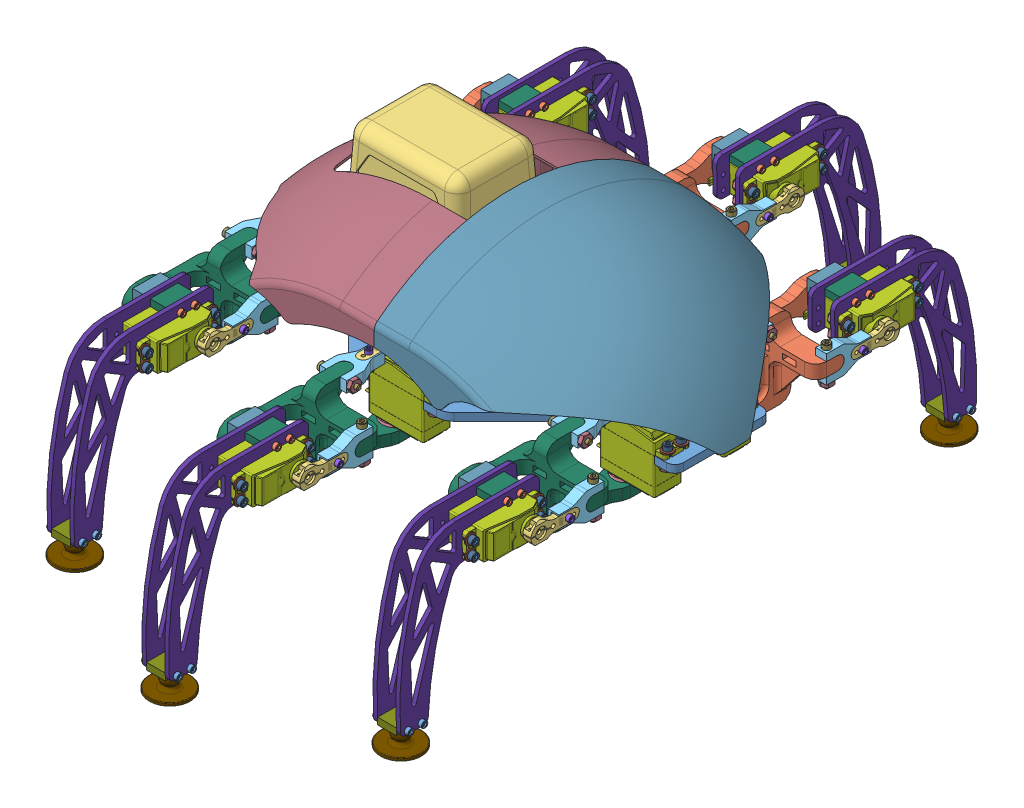
SolidWorks assembly Hexapod_(Small), configuration Défaut. Lengths in mm.
Overall size (338.69 208.02 531.29).
425 component instances, 33 part files, 134 mates.
Components (placement in the parent):
- Body_(Small)-5: Body_(Small) [Default] at (-310 -5.6 15.2) x (1 0 0) z (0 1 0) size (310 170.8 5.6)
- Foot+Femur_(Mirror)-6: Foot+Femur_(Mirror) [Défaut] at (-15 -28 -0.2) x (0 0 1) z (-1 0 0) size (215.83 135.72 63.38)
  - Femur_(Mirror)-1: Femur_(Mirror) [Défaut] at origin size (137.38 61.64 60.79) (flexible)
    - Joint_(Femur_to_tibia)_(Mirror)-2: Joint_(Femur_to_tibia)_(Mirror) [Défaut] at (-66.2306 29.5 32.9516) x (0.999952 0 0.00979) z (-0.00979 0 0.999952) size (122 58.8 58.8)
    - Horn-4: Horn [Défaut] at (-10.2 48.8 30.1) x (-0.999952 0 -0.00979) z (0 1 0) size (35.39 15.87 6)
    - Bearing_mount_(Femur)-2: Bearing_mount_(Femur) [Default] at (2.5 22 30.1) x (1 0 0) z (0 -1 0) size (35.3 20.2 31)
    - Horn_attachment-4: Horn_attachment [Défaut] at (-38.1987 44.8 29.8259) x (0.999952 0 0.00979) z (0 1 0) size (33 20 8)
    - Bearing-4: Bearing [Default] at (-10.2 -6.7498 30.1) x (0.165905 0 -0.986142) z (0.986142 0 0.165905) size (13.87 4.75 13.87)
    - DS3225MG-4: DS3225MG [Default] at (-10.2 45.8 30.1) x (0 0 -1) z (0 1 0) size (57.25 20.4 45.91)
    - HX-SHCS 0.112-40x0.4375x0.4375-N-1: HX-SHCS 0.112-40x0.4375x0.4375-N [HX-SHCS 0.112-40x0.4375x0.4375-N] at (-30.199 51.6448 29.9042) x (0 -1 0) z (-0.508455 0 0.861089) size (13.96 4.65 4.65)
    - MSHXNUT 0.112-40-D-N-1: MSHXNUT 0.112-40-D-N [MSHXNUT 0.112-40-D-N] at (-30.199 40.8 29.9042) x (-0.491498 0 -0.870879) z (0 1 0) size (6.35 7.33 2.49)
    - HX-SHCS 0.138-32x0.5x0.5-N-1: HX-SHCS 0.138-32x0.5x0.5-N [HX-SHCS 0.138-32x0.5x0.5-N] at (-15.2 35.772 -4.7) x (0 -1 0) z (0.866025 0 -0.5) size (16.21 5.74 5.74)
    - Narrow FW 0.138-1: Narrow FW 0.138 [Narrow FW 0.138] at (-15.2 31.2 -4.7) x (0 -1 0) z (-0.829316 0 -0.55878) size (0.81 7.92 7.92)
    - HX-SHCS 0.138-32x0.5x0.5-N-2: HX-SHCS 0.138-32x0.5x0.5-N [HX-SHCS 0.138-32x0.5x0.5-N] at (-15.2 35.772 44.9) x (0 -1 0) z (0.866025 0 -0.5) size (16.21 5.74 5.74)
    - HX-SHCS 0.138-32x0.5x0.5-N-3: HX-SHCS 0.138-32x0.5x0.5-N [HX-SHCS 0.138-32x0.5x0.5-N] at (-5.2 35.772 -4.7) x (0 -1 0) z (0.866025 0 -0.5) size (16.21 5.74 5.74)
    - HX-SHCS 0.138-32x0.5x0.5-N-4: HX-SHCS 0.138-32x0.5x0.5-N [HX-SHCS 0.138-32x0.5x0.5-N] at (-5.2 35.772 44.9) x (0 -1 0) z (0.866025 0 -0.5) size (16.21 5.74 5.74)
    - Narrow FW 0.138-2: Narrow FW 0.138 [Narrow FW 0.138] at (-15.2 31.2 44.9) x (0 -1 0) z (-0.829316 0 -0.55878) size (0.81 7.92 7.92)
    - Narrow FW 0.138-3: Narrow FW 0.138 [Narrow FW 0.138] at (-5.2 31.2 -4.7) x (0 -1 0) z (-0.829316 0 -0.55878) size (0.81 7.92 7.92)
    - Narrow FW 0.138-4: Narrow FW 0.138 [Narrow FW 0.138] at (-5.2 31.2 44.9) x (0 -1 0) z (-0.829316 0 -0.55878) size (0.81 7.92 7.92)
    - HX-SHCS 0.138-32x1x1-N-1: HX-SHCS 0.138-32x1x1-N [HX-SHCS 0.138-32x1x1-N] at (-52.3302 44.8 43.1934) x (0.00979 0 -0.999952) z (-0.865984 0.5 -0.008479) size (28.91 5.74 5.74)
    - MSHXNUT 0.138-32-D-N-1: MSHXNUT 0.138-32-D-N [MSHXNUT 0.138-32-D-N] at (-52.0717 44.8 16.7938) x (0.865984 -0.5 0.008479) z (0.00979 0 -0.999952) size (7.92 9.15 2.9)
  - Foot_(Short)_(Mirror)-1: Foot_(Short)_(Mirror) [Défaut] at (-102.2988 19.1911 38.5987) x (0.999893 -0.010844 0.00979) z (-0.00979 0 0.999952) size (133.45 132 60.64) (flexible)
    - Horn_attachment-2: Horn_attachment [Défaut] at (17.8984 10.5036 -44.8) x (-0.999941 -0.010844 0) z (0 0 -1) size (33 20 8)
    - Bearing-2: Bearing [Default] at (-10.1 10.2 6.7498) x (0.20972 0.977761 0) z (-0.977761 0.20972 0) size (13.87 4.75 13.87)
    - Bearing_mount_(Foot)-2: Bearing_mount_(Foot) [Default] at (-10.1 22.9 -8.1) x (0 1 0) z (0 0 1) size (25.3 20.2 17.1)
    - Link-3: Link [Default] at (-10.1 22.9 -25) x (0 -1 0) z (0 0 1) size (5 20.2 13.9)
    - Horn-2: Horn [Défaut] at (-10.1 10.2 -48.8) x (0.999941 0.010844 0) z (0 0 -1) size (35.39 15.87 6)
    - Joint_(Foot_to_slipper)-4: Joint_(Foot_to_slipper) [Default] at (-82.4457 -87.5 -25) x (0 1 0) z (0 0 1) size (15 20.2 13.9)
    - Foot_(Short)-3: Foot_(Short) [Default] at (-21.5 14 -28) size (102.48 118 3)
    - DS3225MG-2: DS3225MG [Default] at (-10.1 10.2 -45.8) x (-1 0 0) z (0 0 -1) size (57.25 20.4 45.91)
    - Foot_(Short)-4: Foot_(Short) [Default] at (-21.5 14 -11.1) size (102.48 118 3)
    - Slipper-1: Slipper [Défaut] at (-82.4457 -102 -18.05) size (30 10.55 30)
    - HX-SHCS 0.112-40x0.4375x0.4375-N-1: HX-SHCS 0.112-40x0.4375x0.4375-N [HX-SHCS 0.112-40x0.4375x0.4375-N] at (9.8988 10.4169 -51.6448) x (0 0 1) z (0.509362 -0.860552 0) size (13.96 4.65 4.65)
    - MSHXNUT 0.112-40-D-N-1: MSHXNUT 0.112-40-D-N [MSHXNUT 0.112-40-D-N] at (9.8988 10.4169 -40.8) x (-0.509362 0.860552 0) z (0 0 -1) size (6.35 7.33 2.49)
    - HX-SHCS 0.112-40x0.875x0.875-N-1: HX-SHCS 0.112-40x0.875x0.875-N [HX-SHCS 0.112-40x0.875x0.875-N] at (-87.4457 -87.5 -30.8448) x (0 0 1) z (0 1 0) size (25.07 4.65 4.65)
    - MSHXNUT 0.112-40-D-N-2: MSHXNUT 0.112-40-D-N [MSHXNUT 0.112-40-D-N] at (-87.4457 -87.5 -8.1) x (-0.866025 -0.5 0) z (0 0 -1) size (6.35 7.33 2.49)
    - MSHXNUT 0.112-40-D-N-3: MSHXNUT 0.112-40-D-N [MSHXNUT 0.112-40-D-N] at (-77.4457 -87.5 -8.1) x (-0.866025 -0.5 0) z (0 0 -1) size (6.35 7.33 2.49)
    - HX-SHCS 0.112-40x0.875x0.875-N-2: HX-SHCS 0.112-40x0.875x0.875-N [HX-SHCS 0.112-40x0.875x0.875-N] at (-77.4457 -87.5 -30.8448) x (0 0 1) z (0 1 0) size (25.07 4.65 4.65)
    - HX-SHCS 0.112-40x1x0.75-N-3: HX-SHCS 0.112-40x1x0.75-N [HX-SHCS 0.112-40x1x0.75-N] at (-5.1 22.9 -30.8448) x (0 0 1) z (-0.866025 0.5 0) size (28.24 4.65 4.65)
    - HX-SHCS 0.112-40x1x0.75-N-4: HX-SHCS 0.112-40x1x0.75-N [HX-SHCS 0.112-40x1x0.75-N] at (-15.1 22.9 -30.8448) x (0 0 1) z (-0.866025 0.5 0) size (28.24 4.65 4.65)
    - HX-SHCS 0.138-32x0.5x0.5-N-1: HX-SHCS 0.138-32x0.5x0.5-N [HX-SHCS 0.138-32x0.5x0.5-N] at (-44.9 5.2 -35.772) x (0 0 1) z (-0.866025 0.5 0) size (16.21 5.74 5.74)
    - Narrow FW 0.138-1: Narrow FW 0.138 [Narrow FW 0.138] at (-44.9 5.2 -31.2) x (0 0 1) z (0.552023 0.833829 0) size (0.81 7.92 7.92)
    - MSHXNUT 0.138-32-D-N-1: MSHXNUT 0.138-32-D-N [MSHXNUT 0.138-32-D-N] at (-44.9 5.2 -25) x (-0.866025 -0.5 0) z (0 0 -1) size (7.92 9.15 2.9)
    - HX-SHCS 0.138-32x0.5x0.5-N-2: HX-SHCS 0.138-32x0.5x0.5-N [HX-SHCS 0.138-32x0.5x0.5-N] at (4.7 5.2 -35.772) x (0 0 1) z (-0.866025 0.5 0) size (16.21 5.74 5.74)
    - HX-SHCS 0.138-32x0.5x0.5-N-3: HX-SHCS 0.138-32x0.5x0.5-N [HX-SHCS 0.138-32x0.5x0.5-N] at (-44.9 15.2 -35.772) x (0 0 1) z (-0.866025 0.5 0) size (16.21 5.74 5.74)
    - HX-SHCS 0.138-32x0.5x0.5-N-4: HX-SHCS 0.138-32x0.5x0.5-N [HX-SHCS 0.138-32x0.5x0.5-N] at (4.7 15.2 -35.772) x (0 0 1) z (-0.866025 0.5 0) size (16.21 5.74 5.74)
    - Narrow FW 0.138-2: Narrow FW 0.138 [Narrow FW 0.138] at (4.7 5.2 -31.2) x (0 0 1) z (0.552023 0.833829 0) size (0.81 7.92 7.92)
    - Narrow FW 0.138-3: Narrow FW 0.138 [Narrow FW 0.138] at (-44.9 15.2 -31.2) x (0 0 1) z (0.552023 0.833829 0) size (0.81 7.92 7.92)
    - Narrow FW 0.138-4: Narrow FW 0.138 [Narrow FW 0.138] at (4.7 15.2 -31.2) x (0 0 1) z (0.552023 0.833829 0) size (0.81 7.92 7.92)
    - MSHXNUT 0.138-32-D-N-2: MSHXNUT 0.138-32-D-N [MSHXNUT 0.138-32-D-N] at (4.7 5.2 -25) x (-0.866025 -0.5 0) z (0 0 -1) size (7.92 9.15 2.9)
    - MSHXNUT 0.138-32-D-N-3: MSHXNUT 0.138-32-D-N [MSHXNUT 0.138-32-D-N] at (-44.9 15.2 -25) x (-0.866025 -0.5 0) z (0 0 -1) size (7.92 9.15 2.9)
    - MSHXNUT 0.138-32-D-N-4: MSHXNUT 0.138-32-D-N [MSHXNUT 0.138-32-D-N] at (4.7 15.2 -25) x (-0.866025 -0.5 0) z (0 0 -1) size (7.92 9.15 2.9)
  - HX-SHCS 0.138-32x1x1-N-1: HX-SHCS 0.138-32x1x1-N [HX-SHCS 0.138-32x1x1-N] at (-69.8506 43.0052 -5.8857) x (0 -1 0) z (0.861089 0 0.508455) size (28.91 5.74 5.74)
  - MSHXNUT 0.138-32-D-N-1: MSHXNUT 0.138-32-D-N [MSHXNUT 0.138-32-D-N] at (-69.8506 16.6044 -5.8857) x (0.00979 0 -0.999952) z (0 -1 0) size (7.92 9.15 2.9)
- Battery-1: Battery [Défaut] at (-120.5058 65.3901 15.3939) x (0 0 -1) z (-1 0 0) size (64.47 74.3 85.78)
  - MAKITA 4.0AH-1: MAKITA 4.0AH [Défaut] at (0.5853 -29.7874 85.4436) size (64.47 57.15 85.78)
  - MAKITA 4.0AH MOBILE-1: MAKITA 4.0AH MOBILE [Défaut] at (0.5853 -39.3124 91.7936) size (45.84 26.68 66.29)
- arduinoMega-1: arduinoMega [Detailed] at (-199.11 -7.6 14.42) x (0 0 -1) z (-1 0 0) size (108.32 14.5 53.3)
- raspberryPi3B-1: raspberryPi3B [Detailed] at (-109 6.35 15.2) x (-1 0 0) z (0 1 0) size (87.05 58.5 19.5)
- 12Channel PWM-1: 12Channel PWM [Default] at (-145.4 -5.6 15.2) x (-1 0 0) z (0 0 1) size (25.4 7.55 66.7)
- DROK_090483.stp-1: DROK_090483.stp [Default] at (-77.5 -5.6 45.2) x (-1 0 0) z (0 -1 0) size (50.02 60 18.9)
- HX-SHCS 0.138-32x0.625x0.625-N-2: HX-SHCS 0.138-32x0.625x0.625-N [HX-SHCS 0.138-32x0.625x0.625-N] at (-40.288 3.5052 19.69) x (0 -1 0) z (1 0 0) size (19.38 5.74 5.74)
- HX-SHCS 0.138-32x0.625x0.625-N-3: HX-SHCS 0.138-32x0.625x0.625-N [HX-SHCS 0.138-32x0.625x0.625-N] at (-50.288 3.5052 19.69) x (0 -1 0) z (0.5 0 0.866025) size (19.38 5.74 5.74)
- HX-SHCS 0.138-32x0.625x0.625-N-4: HX-SHCS 0.138-32x0.625x0.625-N [HX-SHCS 0.138-32x0.625x0.625-N] at (-50.288 3.5052 10.71) x (0 -1 0) z (1 0 0) size (19.38 5.74 5.74)
- HX-SHCS 0.138-32x0.625x0.625-N-5: HX-SHCS 0.138-32x0.625x0.625-N [HX-SHCS 0.138-32x0.625x0.625-N] at (-40.288 3.5052 10.71) x (0 -1 0) z (1 0 0) size (19.38 5.74 5.74)
- HX-SHCS 0.138-32x0.625x0.625-N-6: HX-SHCS 0.138-32x0.625x0.625-N [HX-SHCS 0.138-32x0.625x0.625-N] at (-170.288 3.5052 69.69) x (0 -1 0) z (1 0 0) size (19.38 5.74 5.74)
- HX-SHCS 0.138-32x0.625x0.625-N-7: HX-SHCS 0.138-32x0.625x0.625-N [HX-SHCS 0.138-32x0.625x0.625-N] at (-160.288 3.5052 69.69) x (0 -1 0) z (1 0 0) size (19.38 5.74 5.74)
- HX-SHCS 0.138-32x0.625x0.625-N-14: HX-SHCS 0.138-32x0.625x0.625-N [HX-SHCS 0.138-32x0.625x0.625-N] at (-160.288 3.5052 -39.29) x (0 -1 0) z (1 0 0) size (19.38 5.74 5.74)
- HX-SHCS 0.138-32x0.625x0.625-N-15: HX-SHCS 0.138-32x0.625x0.625-N [HX-SHCS 0.138-32x0.625x0.625-N] at (-170.288 3.5052 -39.29) x (0 -1 0) z (1 0 0) size (19.38 5.74 5.74)
- HX-SHCS 0.138-32x0.625x0.625-N-16: HX-SHCS 0.138-32x0.625x0.625-N [HX-SHCS 0.138-32x0.625x0.625-N] at (-279.9 3.5052 19.3) x (0 -1 0) z (1 0 0) size (19.38 5.74 5.74)
- HX-SHCS 0.138-32x0.625x0.625-N-17: HX-SHCS 0.138-32x0.625x0.625-N [HX-SHCS 0.138-32x0.625x0.625-N] at (-289.9 3.5052 19.3) x (0 -1 0) z (0.5 0 0.866025) size (19.38 5.74 5.74)
- HX-SHCS 0.138-32x0.625x0.625-N-18: HX-SHCS 0.138-32x0.625x0.625-N [HX-SHCS 0.138-32x0.625x0.625-N] at (-289.9 3.5052 11.1) x (0 -1 0) z (1 0 0) size (19.38 5.74 5.74)
- HX-SHCS 0.138-32x0.625x0.625-N-19: HX-SHCS 0.138-32x0.625x0.625-N [HX-SHCS 0.138-32x0.625x0.625-N] at (-279.9 3.5052 11.1) x (0 -1 0) z (1 0 0) size (19.38 5.74 5.74)
- MSHXNUT 0.138-32-D-N-60: MSHXNUT 0.138-32-D-N [MSHXNUT 0.138-32-D-N] at (-298.75 -8.4956 -15.08) x (1 0 0) z (0 -1 0) size (7.92 9.15 2.9)
- MSHXNUT 0.138-32-D-N-65: MSHXNUT 0.138-32-D-N [MSHXNUT 0.138-32-D-N] at (-298.75 -8.4956 -4.92) x (1 0 0) z (0 -1 0) size (7.92 9.15 2.9)
- MSHXNUT 0.138-32-D-N-70: MSHXNUT 0.138-32-D-N [MSHXNUT 0.138-32-D-N] at (-251.252 -8.4956 -4.92) x (0.5 0 0.866025) z (0 -1 0) size (7.92 9.15 2.9)
- MSHXNUT 0.138-32-D-N-75: MSHXNUT 0.138-32-D-N [MSHXNUT 0.138-32-D-N] at (-251.252 -8.4956 -15.08) x (0.5 0 0.866025) z (0 -1 0) size (7.92 9.15 2.9)
- MSHXNUT 0.138-32-D-N-80: MSHXNUT 0.138-32-D-N [MSHXNUT 0.138-32-D-N] at (-279.9 -13.5656 11.1) x (0 0 1) z (0 -1 0) size (7.92 9.15 2.9)
- MSHXNUT 0.138-32-D-N-85: MSHXNUT 0.138-32-D-N [MSHXNUT 0.138-32-D-N] at (-289.9 -13.5656 11.1) x (0 0 1) z (0 -1 0) size (7.92 9.15 2.9)
- MSHXNUT 0.138-32-D-N-88: MSHXNUT 0.138-32-D-N [MSHXNUT 0.138-32-D-N] at (-178.75 -8.4956 -65.08) x (1 0 0) z (0 -1 0) size (7.92 9.15 2.9)
- MSHXNUT 0.138-32-D-N-89: MSHXNUT 0.138-32-D-N [MSHXNUT 0.138-32-D-N] at (-178.75 -8.4956 -54.92) x (1 0 0) z (0 -1 0) size (7.92 9.15 2.9)
- MSHXNUT 0.138-32-D-N-90: MSHXNUT 0.138-32-D-N [MSHXNUT 0.138-32-D-N] at (-131.252 -8.4956 -54.92) x (0.5 0 0.866025) z (0 -1 0) size (7.92 9.15 2.9)
- MSHXNUT 0.138-32-D-N-91: MSHXNUT 0.138-32-D-N [MSHXNUT 0.138-32-D-N] at (-131.252 -8.4956 -65.08) x (0.5 0 0.866025) z (0 -1 0) size (7.92 9.15 2.9)
- MSHXNUT 0.138-32-D-N-92: MSHXNUT 0.138-32-D-N [MSHXNUT 0.138-32-D-N] at (-159.9 -13.5656 -38.9) x (0 0 1) z (0 -1 0) size (7.92 9.15 2.9)
- MSHXNUT 0.138-32-D-N-93: MSHXNUT 0.138-32-D-N [MSHXNUT 0.138-32-D-N] at (-169.9 -13.5656 -38.9) x (0 0 1) z (0 -1 0) size (7.92 9.15 2.9)
- MSHXNUT 0.138-32-D-N-94: MSHXNUT 0.138-32-D-N [MSHXNUT 0.138-32-D-N] at (-49.9 -13.5656 11.1) x (0 0 1) z (0 -1 0) size (7.92 9.15 2.9)
- MSHXNUT 0.138-32-D-N-95: MSHXNUT 0.138-32-D-N [MSHXNUT 0.138-32-D-N] at (-39.9 -13.5656 11.1) x (0 0 1) z (0 -1 0) size (7.92 9.15 2.9)
- MSHXNUT 0.138-32-D-N-96: MSHXNUT 0.138-32-D-N [MSHXNUT 0.138-32-D-N] at (-11.252 -8.4956 -4.92) x (0.5 0 0.866025) z (0 -1 0) size (7.92 9.15 2.9)
- MSHXNUT 0.138-32-D-N-97: MSHXNUT 0.138-32-D-N [MSHXNUT 0.138-32-D-N] at (-11.252 -8.4956 -15.08) x (0.5 0 0.866025) z (0 -1 0) size (7.92 9.15 2.9)
- MSHXNUT 0.138-32-D-N-98: MSHXNUT 0.138-32-D-N [MSHXNUT 0.138-32-D-N] at (-58.75 -8.4956 -4.92) x (1 0 0) z (0 -1 0) size (7.92 9.15 2.9)
- MSHXNUT 0.138-32-D-N-99: MSHXNUT 0.138-32-D-N [MSHXNUT 0.138-32-D-N] at (-58.75 -8.4956 -15.08) x (1 0 0) z (0 -1 0) size (7.92 9.15 2.9)
- MSHXNUT 0.138-32-D-N-100: MSHXNUT 0.138-32-D-N [MSHXNUT 0.138-32-D-N] at (-289.9 -10.67 19.3) x (0 0 -1) z (0 1 0) size (7.92 9.15 2.9)
- MSHXNUT 0.138-32-D-N-101: MSHXNUT 0.138-32-D-N [MSHXNUT 0.138-32-D-N] at (-279.9 -10.67 19.3) x (0 0 -1) z (0 1 0) size (7.92 9.15 2.9)
- MSHXNUT 0.138-32-D-N-102: MSHXNUT 0.138-32-D-N [MSHXNUT 0.138-32-D-N] at (-251.252 -5.6 35.32) x (0.5 0 -0.866025) z (0 1 0) size (7.92 9.15 2.9)
- MSHXNUT 0.138-32-D-N-103: MSHXNUT 0.138-32-D-N [MSHXNUT 0.138-32-D-N] at (-251.252 -5.6 45.48) x (0.5 0 -0.866025) z (0 1 0) size (7.92 9.15 2.9)
- MSHXNUT 0.138-32-D-N-104: MSHXNUT 0.138-32-D-N [MSHXNUT 0.138-32-D-N] at (-298.75 -5.6 35.32) x (1 0 0) z (0 1 0) size (7.92 9.15 2.9)
- MSHXNUT 0.138-32-D-N-105: MSHXNUT 0.138-32-D-N [MSHXNUT 0.138-32-D-N] at (-298.75 -5.6 45.48) x (1 0 0) z (0 1 0) size (7.92 9.15 2.9)
- MSHXNUT 0.138-32-D-N-106: MSHXNUT 0.138-32-D-N [MSHXNUT 0.138-32-D-N] at (-178.75 -5.6 95.48) x (1 0 0) z (0 1 0) size (7.92 9.15 2.9)
- MSHXNUT 0.138-32-D-N-107: MSHXNUT 0.138-32-D-N [MSHXNUT 0.138-32-D-N] at (-178.75 -5.6 85.32) x (1 0 0) z (0 1 0) size (7.92 9.15 2.9)
- MSHXNUT 0.138-32-D-N-108: MSHXNUT 0.138-32-D-N [MSHXNUT 0.138-32-D-N] at (-131.252 -5.6 85.32) x (0.5 0 -0.866025) z (0 1 0) size (7.92 9.15 2.9)
- MSHXNUT 0.138-32-D-N-109: MSHXNUT 0.138-32-D-N [MSHXNUT 0.138-32-D-N] at (-131.252 -5.6 95.48) x (0.5 0 -0.866025) z (0 1 0) size (7.92 9.15 2.9)
- MSHXNUT 0.138-32-D-N-110: MSHXNUT 0.138-32-D-N [MSHXNUT 0.138-32-D-N] at (-159.9 -10.67 69.3) x (0 0 -1) z (0 1 0) size (7.92 9.15 2.9)
- MSHXNUT 0.138-32-D-N-111: MSHXNUT 0.138-32-D-N [MSHXNUT 0.138-32-D-N] at (-169.9 -10.67 69.3) x (0 0 -1) z (0 1 0) size (7.92 9.15 2.9)
- MSHXNUT 0.138-32-D-N-112: MSHXNUT 0.138-32-D-N [MSHXNUT 0.138-32-D-N] at (-49.9 -10.67 19.3) x (0 0 -1) z (0 1 0) size (7.92 9.15 2.9)
- MSHXNUT 0.138-32-D-N-113: MSHXNUT 0.138-32-D-N [MSHXNUT 0.138-32-D-N] at (-39.9 -10.67 19.3) x (0 0 -1) z (0 1 0) size (7.92 9.15 2.9)
- MSHXNUT 0.138-32-D-N-114: MSHXNUT 0.138-32-D-N [MSHXNUT 0.138-32-D-N] at (-11.252 -5.6 35.32) x (0.5 0 -0.866025) z (0 1 0) size (7.92 9.15 2.9)
- MSHXNUT 0.138-32-D-N-115: MSHXNUT 0.138-32-D-N [MSHXNUT 0.138-32-D-N] at (-11.252 -5.6 45.48) x (0.5 0 -0.866025) z (0 1 0) size (7.92 9.15 2.9)
- MSHXNUT 0.138-32-D-N-116: MSHXNUT 0.138-32-D-N [MSHXNUT 0.138-32-D-N] at (-58.75 -5.6 35.32) x (1 0 0) z (0 1 0) size (7.92 9.15 2.9)
- MSHXNUT 0.138-32-D-N-117: MSHXNUT 0.138-32-D-N [MSHXNUT 0.138-32-D-N] at (-58.75 -5.6 45.48) x (1 0 0) z (0 1 0) size (7.92 9.15 2.9)
- HX-SHCS 0.138-32x0.5x0.5-N-20: HX-SHCS 0.138-32x0.5x0.5-N [HX-SHCS 0.138-32x0.5x0.5-N] at (-175 -12.6052 48.68) x (0 1 0) z (-0.5 0 -0.866025) size (16.21 5.74 5.74)
- HX-SHCS 0.138-32x0.5x0.5-N-21: HX-SHCS 0.138-32x0.5x0.5-N [HX-SHCS 0.138-32x0.5x0.5-N] at (-223.22 -12.6052 -32.56) x (0 1 0) z (1 0 0) size (16.21 5.74 5.74)
- HX-SHCS 0.138-32x0.5x0.5-N-22: HX-SHCS 0.138-32x0.5x0.5-N [HX-SHCS 0.138-32x0.5x0.5-N] at (-175 -12.6052 -26.2) x (0 1 0) z (-0.5 0 -0.866025) size (16.21 5.74 5.74)
- HX-SHCS 0.138-32x0.5x0.5-N-23: HX-SHCS 0.138-32x0.5x0.5-N [HX-SHCS 0.138-32x0.5x0.5-N] at (-223.22 -12.6052 49.91) x (0 1 0) z (-1 0 0) size (16.21 5.74 5.74)
- MSHXNUT 0.112-40-D-N-106: MSHXNUT 0.112-40-D-N [MSHXNUT 0.112-40-D-N] at (-223.22 2.4892 -32.56) x (1 0 0) z (0 1 0) size (6.35 7.33 2.49)
- MSHXNUT 0.112-40-D-N-107: MSHXNUT 0.112-40-D-N [MSHXNUT 0.112-40-D-N] at (-223.22 2.4892 49.91) x (1 0 0) z (0 1 0) size (6.35 7.33 2.49)
- MSHXNUT 0.112-40-D-N-108: MSHXNUT 0.112-40-D-N [MSHXNUT 0.112-40-D-N] at (-175 2.4892 -26.2) x (1 0 0) z (0 1 0) size (6.35 7.33 2.49)
- MSHXNUT 0.112-40-D-N-109: MSHXNUT 0.112-40-D-N [MSHXNUT 0.112-40-D-N] at (-175 2.4892 48.68) x (1 0 0) z (0 1 0) size (6.35 7.33 2.49)
- HX-SHCS 0.138-32x0.5x0.5-N-24: HX-SHCS 0.138-32x0.5x0.5-N [HX-SHCS 0.138-32x0.5x0.5-N] at (-117.315 -10.3052 -11.215) x (0 1 0) z (-0.5 0 -0.866025) size (16.21 5.74 5.74)
- MSHXNUT 0.112-40-D-N-110: MSHXNUT 0.112-40-D-N [MSHXNUT 0.112-40-D-N] at (-117.315 2.4892 -11.215) x (1 0 0) z (0 1 0) size (6.35 7.33 2.49)
- HX-SHCS 0.138-32x0.5x0.5-N-28: HX-SHCS 0.138-32x0.5x0.5-N [HX-SHCS 0.138-32x0.5x0.5-N] at (-80.685 -10.3052 -11.215) x (0 1 0) z (-0.5 0 -0.866025) size (16.21 5.74 5.74)
- HX-SHCS 0.138-32x0.5x0.5-N-29: HX-SHCS 0.138-32x0.5x0.5-N [HX-SHCS 0.138-32x0.5x0.5-N] at (-117.315 -10.3052 41.615) x (0 1 0) z (-0.5 0 -0.866025) size (16.21 5.74 5.74)
- HX-SHCS 0.138-32x0.5x0.5-N-30: HX-SHCS 0.138-32x0.5x0.5-N [HX-SHCS 0.138-32x0.5x0.5-N] at (-80.685 -10.3052 41.615) x (0 1 0) z (-0.5 0 -0.866025) size (16.21 5.74 5.74)
- MSHXNUT 0.112-40-D-N-114: MSHXNUT 0.112-40-D-N [MSHXNUT 0.112-40-D-N] at (-80.685 2.4892 -11.215) x (1 0 0) z (0 1 0) size (6.35 7.33 2.49)
- MSHXNUT 0.112-40-D-N-115: MSHXNUT 0.112-40-D-N [MSHXNUT 0.112-40-D-N] at (-117.315 2.4892 41.615) x (1 0 0) z (0 1 0) size (6.35 7.33 2.49)
- MSHXNUT 0.112-40-D-N-116: MSHXNUT 0.112-40-D-N [MSHXNUT 0.112-40-D-N] at (-80.685 2.4892 41.615) x (1 0 0) z (0 1 0) size (6.35 7.33 2.49)
- 1_4_Round_Aluminum_Standoff.step-1: 1_4_Round_Aluminum_Standoff.step [Défaut] at (-70 0 -9.3) x (0.963282 0 -0.268492) z (0.268492 0 0.963282) size (6.34 6.36 6.34)
- HX-SHCS 0.112-40x1x0.75-N-47: HX-SHCS 0.112-40x1x0.75-N [HX-SHCS 0.112-40x1x0.75-N] at (-70 10.4948 -9.3) x (0 -1 0) z (0.637638 0 0.770336) size (28.24 4.65 4.65)
- MSHXNUT 0.112-40-D-N-117: MSHXNUT 0.112-40-D-N [MSHXNUT 0.112-40-D-N] at (-70 -8.0892 -9.3) x (1 0 0) z (0 -1 0) size (6.35 7.33 2.49)
- 1_4_Round_Aluminum_Standoff.step-2: 1_4_Round_Aluminum_Standoff.step [Défaut] at (-128 0 -9.3) x (0.963282 0 -0.268492) z (0.268492 0 0.963282) size (6.34 6.36 6.34)
- 1_4_Round_Aluminum_Standoff.step-3: 1_4_Round_Aluminum_Standoff.step [Défaut] at (-70 0 39.7) x (0.963282 0 -0.268492) z (0.268492 0 0.963282) size (6.34 6.36 6.34)
- 1_4_Round_Aluminum_Standoff.step-4: 1_4_Round_Aluminum_Standoff.step [Défaut] at (-128 0 39.7) x (0.963282 0 -0.268492) z (0.268492 0 0.963282) size (6.34 6.36 6.34)
- MSHXNUT 0.112-40-D-N-121: MSHXNUT 0.112-40-D-N [MSHXNUT 0.112-40-D-N] at (-128 -8.0892 -9.3) x (1 0 0) z (0 -1 0) size (6.35 7.33 2.49)
- MSHXNUT 0.112-40-D-N-122: MSHXNUT 0.112-40-D-N [MSHXNUT 0.112-40-D-N] at (-70 -8.0892 39.7) x (1 0 0) z (0 -1 0) size (6.35 7.33 2.49)
- MSHXNUT 0.112-40-D-N-123: MSHXNUT 0.112-40-D-N [MSHXNUT 0.112-40-D-N] at (-128 -8.0892 39.7) x (1 0 0) z (0 -1 0) size (6.35 7.33 2.49)
- HX-SHCS 0.112-40x1x0.75-N-51: HX-SHCS 0.112-40x1x0.75-N [HX-SHCS 0.112-40x1x0.75-N] at (-128 10.4948 -9.3) x (0 -1 0) z (0.637638 0 0.770336) size (28.24 4.65 4.65)
- HX-SHCS 0.112-40x1x0.75-N-52: HX-SHCS 0.112-40x1x0.75-N [HX-SHCS 0.112-40x1x0.75-N] at (-70 10.4948 39.7) x (0 -1 0) z (0.637638 0 0.770336) size (28.24 4.65 4.65)
- HX-SHCS 0.112-40x1x0.75-N-53: HX-SHCS 0.112-40x1x0.75-N [HX-SHCS 0.112-40x1x0.75-N] at (-128 10.4948 39.7) x (0 -1 0) z (0.637638 0 0.770336) size (28.24 4.65 4.65)
- HX-SHCS 0.112-40x0.5x0.5-N-32: HX-SHCS 0.112-40x0.5x0.5-N [HX-SHCS 0.112-40x0.5x0.5-N] at (-154.8 -9.9448 -12.75) x (0 1 0) z (-1 0 0) size (15.54 4.65 4.65)
- MSHXNUT 0.112-40-D-N-124: MSHXNUT 0.112-40-D-N [MSHXNUT 0.112-40-D-N] at (-154.8 2.4892 -12.75) x (1 0 0) z (0 1 0) size (6.35 7.33 2.49)
- HX-SHCS 0.112-40x0.5x0.5-N-36: HX-SHCS 0.112-40x0.5x0.5-N [HX-SHCS 0.112-40x0.5x0.5-N] at (-136 -9.9448 -12.75) x (0 1 0) z (-1 0 0) size (15.54 4.65 4.65)
- HX-SHCS 0.112-40x0.5x0.5-N-37: HX-SHCS 0.112-40x0.5x0.5-N [HX-SHCS 0.112-40x0.5x0.5-N] at (-154.8 -9.9448 43.15) x (0 1 0) z (-1 0 0) size (15.54 4.65 4.65)
- HX-SHCS 0.112-40x0.5x0.5-N-38: HX-SHCS 0.112-40x0.5x0.5-N [HX-SHCS 0.112-40x0.5x0.5-N] at (-136 -9.9448 43.15) x (0 1 0) z (-1 0 0) size (15.54 4.65 4.65)
- MSHXNUT 0.112-40-D-N-128: MSHXNUT 0.112-40-D-N [MSHXNUT 0.112-40-D-N] at (-136 2.4892 -12.75) x (1 0 0) z (0 1 0) size (6.35 7.33 2.49)
- MSHXNUT 0.112-40-D-N-129: MSHXNUT 0.112-40-D-N [MSHXNUT 0.112-40-D-N] at (-154.8 2.4892 43.15) x (1 0 0) z (0 1 0) size (6.35 7.33 2.49)
- MSHXNUT 0.112-40-D-N-130: MSHXNUT 0.112-40-D-N [MSHXNUT 0.112-40-D-N] at (-136 2.4892 43.15) x (1 0 0) z (0 1 0) size (6.35 7.33 2.49)
- 1_4_Round_Aluminum_Standoff.step-5: 1_4_Round_Aluminum_Standoff.step [Défaut] at (-182.4233 0 -9.675) x (0.963282 0 -0.268492) z (0.268492 0 0.963282) size (6.34 6.36 6.34)
- 1_4_Round_Aluminum_Standoff.step-6: 1_4_Round_Aluminum_Standoff.step [Défaut] at (-182.4233 0 39.675) x (0.963282 0 -0.268492) z (0.268492 0 0.963282) size (6.34 6.36 6.34)
- 1_4_Round_Aluminum_Standoff.step-7: 1_4_Round_Aluminum_Standoff.step [Défaut] at (-231.7733 0 -9.675) x (0.963282 0 -0.268492) z (0.268492 0 0.963282) size (6.34 6.36 6.34)
- 1_4_Round_Aluminum_Standoff.step-8: 1_4_Round_Aluminum_Standoff.step [Défaut] at (-231.7733 0 39.675) x (0.963282 0 -0.268492) z (0.268492 0 0.963282) size (6.34 6.36 6.34)
- HX-SHCS 0.112-40x1x0.75-N-61: HX-SHCS 0.112-40x1x0.75-N [HX-SHCS 0.112-40x1x0.75-N] at (-182.4233 -8.4448 -9.675) x (0 1 0) z (0.993964 0 -0.109708) size (28.24 4.65 4.65)
- HX-SHCS 0.112-40x1x0.75-N-62: HX-SHCS 0.112-40x1x0.75-N [HX-SHCS 0.112-40x1x0.75-N] at (-182.4233 -8.4448 39.675) x (0 1 0) z (0.993964 0 -0.109708) size (28.24 4.65 4.65)
- HX-SHCS 0.112-40x1x0.75-N-63: HX-SHCS 0.112-40x1x0.75-N [HX-SHCS 0.112-40x1x0.75-N] at (-231.7733 -8.4448 -9.675) x (0 1 0) z (0.993964 0 -0.109708) size (28.24 4.65 4.65)
- HX-SHCS 0.112-40x1x0.75-N-64: HX-SHCS 0.112-40x1x0.75-N [HX-SHCS 0.112-40x1x0.75-N] at (-231.7733 -8.4448 39.675) x (0 1 0) z (0.993964 0 -0.109708) size (28.24 4.65 4.65)
- Battery_holder-1: Battery_holder [Default] at (-207.0983 17.7 15) size (60 19.6 60)
- MSHXNUT 0.112-40-D-N-131: MSHXNUT 0.112-40-D-N [MSHXNUT 0.112-40-D-N] at (-182.4233 12.7 -9.675) x (-0.837169 0 -0.546944) z (0 -1 0) size (6.35 7.33 2.49)
- MSHXNUT 0.112-40-D-N-135: MSHXNUT 0.112-40-D-N [MSHXNUT 0.112-40-D-N] at (-182.4233 12.7 39.675) x (-0.837169 0 -0.546944) z (0 -1 0) size (6.35 7.33 2.49)
- MSHXNUT 0.112-40-D-N-136: MSHXNUT 0.112-40-D-N [MSHXNUT 0.112-40-D-N] at (-231.7733 12.7 -9.675) x (-0.837169 0 -0.546944) z (0 -1 0) size (6.35 7.33 2.49)
- MSHXNUT 0.112-40-D-N-137: MSHXNUT 0.112-40-D-N [MSHXNUT 0.112-40-D-N] at (-231.7733 12.7 39.675) x (-0.837169 0 -0.546944) z (0 -1 0) size (6.35 7.33 2.49)
- Shell_(Front)-4: Shell_(Front) [Default] at (-155 -76.2 15.2) x (0 0 1) z (-1 0 0) size (204.71 79.03 165.14)
- Shell_(Back)-3: Shell_(Back) [Default] at (-155 -76.2 15.2) x (0 0 -1) z (1 0 0) size (205.09 91.22 173.55)
- Foot+Femur_(Mirror)-7: Foot+Femur_(Mirror) [Défaut] at (-135 -28 -50.2) x (0 0 1) z (-1 0 0) size (215.83 135.72 63.38)
  - Femur_(Mirror)-1: Femur_(Mirror) [Défaut] at origin size (137.38 61.64 60.79) (flexible)
    - Joint_(Femur_to_tibia)_(Mirror)-2: Joint_(Femur_to_tibia)_(Mirror) [Défaut] at (-66.2306 29.5 32.9516) x (0.999952 0 0.00979) z (-0.00979 0 0.999952) size (122 58.8 58.8)
    - Horn-4: Horn [Défaut] at (-10.2 48.8 30.1) x (-0.999952 0 -0.00979) z (0 1 0) size (35.39 15.87 6)
    - Bearing_mount_(Femur)-2: Bearing_mount_(Femur) [Default] at (2.5 22 30.1) x (1 0 0) z (0 -1 0) size (35.3 20.2 31)
    - Horn_attachment-4: Horn_attachment [Défaut] at (-38.1987 44.8 29.8259) x (0.999952 0 0.00979) z (0 1 0) size (33 20 8)
    - Bearing-4: Bearing [Default] at (-10.2 -6.7498 30.1) x (0.165905 0 -0.986142) z (0.986142 0 0.165905) size (13.87 4.75 13.87)
    - DS3225MG-4: DS3225MG [Default] at (-10.2 45.8 30.1) x (0 0 -1) z (0 1 0) size (57.25 20.4 45.91)
    - HX-SHCS 0.112-40x0.4375x0.4375-N-1: HX-SHCS 0.112-40x0.4375x0.4375-N [HX-SHCS 0.112-40x0.4375x0.4375-N] at (-30.199 51.6448 29.9042) x (0 -1 0) z (-0.508455 0 0.861089) size (13.96 4.65 4.65)
    - MSHXNUT 0.112-40-D-N-1: MSHXNUT 0.112-40-D-N [MSHXNUT 0.112-40-D-N] at (-30.199 40.8 29.9042) x (-0.491498 0 -0.870879) z (0 1 0) size (6.35 7.33 2.49)
    - HX-SHCS 0.138-32x0.5x0.5-N-1: HX-SHCS 0.138-32x0.5x0.5-N [HX-SHCS 0.138-32x0.5x0.5-N] at (-15.2 35.772 -4.7) x (0 -1 0) z (0.866025 0 -0.5) size (16.21 5.74 5.74)
    - Narrow FW 0.138-1: Narrow FW 0.138 [Narrow FW 0.138] at (-15.2 31.2 -4.7) x (0 -1 0) z (-0.829316 0 -0.55878) size (0.81 7.92 7.92)
    - HX-SHCS 0.138-32x0.5x0.5-N-2: HX-SHCS 0.138-32x0.5x0.5-N [HX-SHCS 0.138-32x0.5x0.5-N] at (-15.2 35.772 44.9) x (0 -1 0) z (0.866025 0 -0.5) size (16.21 5.74 5.74)
    - HX-SHCS 0.138-32x0.5x0.5-N-3: HX-SHCS 0.138-32x0.5x0.5-N [HX-SHCS 0.138-32x0.5x0.5-N] at (-5.2 35.772 -4.7) x (0 -1 0) z (0.866025 0 -0.5) size (16.21 5.74 5.74)
    - HX-SHCS 0.138-32x0.5x0.5-N-4: HX-SHCS 0.138-32x0.5x0.5-N [HX-SHCS 0.138-32x0.5x0.5-N] at (-5.2 35.772 44.9) x (0 -1 0) z (0.866025 0 -0.5) size (16.21 5.74 5.74)
    - Narrow FW 0.138-2: Narrow FW 0.138 [Narrow FW 0.138] at (-15.2 31.2 44.9) x (0 -1 0) z (-0.829316 0 -0.55878) size (0.81 7.92 7.92)
    - Narrow FW 0.138-3: Narrow FW 0.138 [Narrow FW 0.138] at (-5.2 31.2 -4.7) x (0 -1 0) z (-0.829316 0 -0.55878) size (0.81 7.92 7.92)
    - Narrow FW 0.138-4: Narrow FW 0.138 [Narrow FW 0.138] at (-5.2 31.2 44.9) x (0 -1 0) z (-0.829316 0 -0.55878) size (0.81 7.92 7.92)
    - HX-SHCS 0.138-32x1x1-N-1: HX-SHCS 0.138-32x1x1-N [HX-SHCS 0.138-32x1x1-N] at (-52.3302 44.8 43.1934) x (0.00979 0 -0.999952) z (-0.865984 0.5 -0.008479) size (28.91 5.74 5.74)
    - MSHXNUT 0.138-32-D-N-1: MSHXNUT 0.138-32-D-N [MSHXNUT 0.138-32-D-N] at (-52.0717 44.8 16.7938) x (0.865984 -0.5 0.008479) z (0.00979 0 -0.999952) size (7.92 9.15 2.9)
  - Foot_(Short)_(Mirror)-1: Foot_(Short)_(Mirror) [Défaut] at (-102.2988 19.1911 38.5987) x (0.999893 -0.010844 0.00979) z (-0.00979 0 0.999952) size (133.45 132 60.64) (flexible)
    - Horn_attachment-2: Horn_attachment [Défaut] at (17.8984 10.5036 -44.8) x (-0.999941 -0.010844 0) z (0 0 -1) size (33 20 8)
    - Bearing-2: Bearing [Default] at (-10.1 10.2 6.7498) x (0.20972 0.977761 0) z (-0.977761 0.20972 0) size (13.87 4.75 13.87)
    - Bearing_mount_(Foot)-2: Bearing_mount_(Foot) [Default] at (-10.1 22.9 -8.1) x (0 1 0) z (0 0 1) size (25.3 20.2 17.1)
    - Link-3: Link [Default] at (-10.1 22.9 -25) x (0 -1 0) z (0 0 1) size (5 20.2 13.9)
    - Horn-2: Horn [Défaut] at (-10.1 10.2 -48.8) x (0.999941 0.010844 0) z (0 0 -1) size (35.39 15.87 6)
    - Joint_(Foot_to_slipper)-4: Joint_(Foot_to_slipper) [Default] at (-82.4457 -87.5 -25) x (0 1 0) z (0 0 1) size (15 20.2 13.9)
    - Foot_(Short)-3: Foot_(Short) [Default] at (-21.5 14 -28) size (102.48 118 3)
    - DS3225MG-2: DS3225MG [Default] at (-10.1 10.2 -45.8) x (-1 0 0) z (0 0 -1) size (57.25 20.4 45.91)
    - Foot_(Short)-4: Foot_(Short) [Default] at (-21.5 14 -11.1) size (102.48 118 3)
    - Slipper-1: Slipper [Défaut] at (-82.4457 -102 -18.05) size (30 10.55 30)
    - HX-SHCS 0.112-40x0.4375x0.4375-N-1: HX-SHCS 0.112-40x0.4375x0.4375-N [HX-SHCS 0.112-40x0.4375x0.4375-N] at (9.8988 10.4169 -51.6448) x (0 0 1) z (0.509362 -0.860552 0) size (13.96 4.65 4.65)
    - MSHXNUT 0.112-40-D-N-1: MSHXNUT 0.112-40-D-N [MSHXNUT 0.112-40-D-N] at (9.8988 10.4169 -40.8) x (-0.509362 0.860552 0) z (0 0 -1) size (6.35 7.33 2.49)
    - HX-SHCS 0.112-40x0.875x0.875-N-1: HX-SHCS 0.112-40x0.875x0.875-N [HX-SHCS 0.112-40x0.875x0.875-N] at (-87.4457 -87.5 -30.8448) x (0 0 1) z (0 1 0) size (25.07 4.65 4.65)
    - MSHXNUT 0.112-40-D-N-2: MSHXNUT 0.112-40-D-N [MSHXNUT 0.112-40-D-N] at (-87.4457 -87.5 -8.1) x (-0.866025 -0.5 0) z (0 0 -1) size (6.35 7.33 2.49)
    - MSHXNUT 0.112-40-D-N-3: MSHXNUT 0.112-40-D-N [MSHXNUT 0.112-40-D-N] at (-77.4457 -87.5 -8.1) x (-0.866025 -0.5 0) z (0 0 -1) size (6.35 7.33 2.49)
    - HX-SHCS 0.112-40x0.875x0.875-N-2: HX-SHCS 0.112-40x0.875x0.875-N [HX-SHCS 0.112-40x0.875x0.875-N] at (-77.4457 -87.5 -30.8448) x (0 0 1) z (0 1 0) size (25.07 4.65 4.65)
    - HX-SHCS 0.112-40x1x0.75-N-3: HX-SHCS 0.112-40x1x0.75-N [HX-SHCS 0.112-40x1x0.75-N] at (-5.1 22.9 -30.8448) x (0 0 1) z (-0.866025 0.5 0) size (28.24 4.65 4.65)
    - HX-SHCS 0.112-40x1x0.75-N-4: HX-SHCS 0.112-40x1x0.75-N [HX-SHCS 0.112-40x1x0.75-N] at (-15.1 22.9 -30.8448) x (0 0 1) z (-0.866025 0.5 0) size (28.24 4.65 4.65)
    - HX-SHCS 0.138-32x0.5x0.5-N-1: HX-SHCS 0.138-32x0.5x0.5-N [HX-SHCS 0.138-32x0.5x0.5-N] at (-44.9 5.2 -35.772) x (0 0 1) z (-0.866025 0.5 0) size (16.21 5.74 5.74)
    - Narrow FW 0.138-1: Narrow FW 0.138 [Narrow FW 0.138] at (-44.9 5.2 -31.2) x (0 0 1) z (0.552023 0.833829 0) size (0.81 7.92 7.92)
    - MSHXNUT 0.138-32-D-N-1: MSHXNUT 0.138-32-D-N [MSHXNUT 0.138-32-D-N] at (-44.9 5.2 -25) x (-0.866025 -0.5 0) z (0 0 -1) size (7.92 9.15 2.9)
    - HX-SHCS 0.138-32x0.5x0.5-N-2: HX-SHCS 0.138-32x0.5x0.5-N [HX-SHCS 0.138-32x0.5x0.5-N] at (4.7 5.2 -35.772) x (0 0 1) z (-0.866025 0.5 0) size (16.21 5.74 5.74)
    - HX-SHCS 0.138-32x0.5x0.5-N-3: HX-SHCS 0.138-32x0.5x0.5-N [HX-SHCS 0.138-32x0.5x0.5-N] at (-44.9 15.2 -35.772) x (0 0 1) z (-0.866025 0.5 0) size (16.21 5.74 5.74)
    - HX-SHCS 0.138-32x0.5x0.5-N-4: HX-SHCS 0.138-32x0.5x0.5-N [HX-SHCS 0.138-32x0.5x0.5-N] at (4.7 15.2 -35.772) x (0 0 1) z (-0.866025 0.5 0) size (16.21 5.74 5.74)
    - Narrow FW 0.138-2: Narrow FW 0.138 [Narrow FW 0.138] at (4.7 5.2 -31.2) x (0 0 1) z (0.552023 0.833829 0) size (0.81 7.92 7.92)
    - Narrow FW 0.138-3: Narrow FW 0.138 [Narrow FW 0.138] at (-44.9 15.2 -31.2) x (0 0 1) z (0.552023 0.833829 0) size (0.81 7.92 7.92)
    - Narrow FW 0.138-4: Narrow FW 0.138 [Narrow FW 0.138] at (4.7 15.2 -31.2) x (0 0 1) z (0.552023 0.833829 0) size (0.81 7.92 7.92)
    - MSHXNUT 0.138-32-D-N-2: MSHXNUT 0.138-32-D-N [MSHXNUT 0.138-32-D-N] at (4.7 5.2 -25) x (-0.866025 -0.5 0) z (0 0 -1) size (7.92 9.15 2.9)
    - MSHXNUT 0.138-32-D-N-3: MSHXNUT 0.138-32-D-N [MSHXNUT 0.138-32-D-N] at (-44.9 15.2 -25) x (-0.866025 -0.5 0) z (0 0 -1) size (7.92 9.15 2.9)
    - MSHXNUT 0.138-32-D-N-4: MSHXNUT 0.138-32-D-N [MSHXNUT 0.138-32-D-N] at (4.7 15.2 -25) x (-0.866025 -0.5 0) z (0 0 -1) size (7.92 9.15 2.9)
  - HX-SHCS 0.138-32x1x1-N-1: HX-SHCS 0.138-32x1x1-N [HX-SHCS 0.138-32x1x1-N] at (-69.8506 43.0052 -5.8857) x (0 -1 0) z (0.861089 0 0.508455) size (28.91 5.74 5.74)
  - MSHXNUT 0.138-32-D-N-1: MSHXNUT 0.138-32-D-N [MSHXNUT 0.138-32-D-N] at (-69.8506 16.6044 -5.8857) x (0.00979 0 -0.999952) z (0 -1 0) size (7.92 9.15 2.9)
